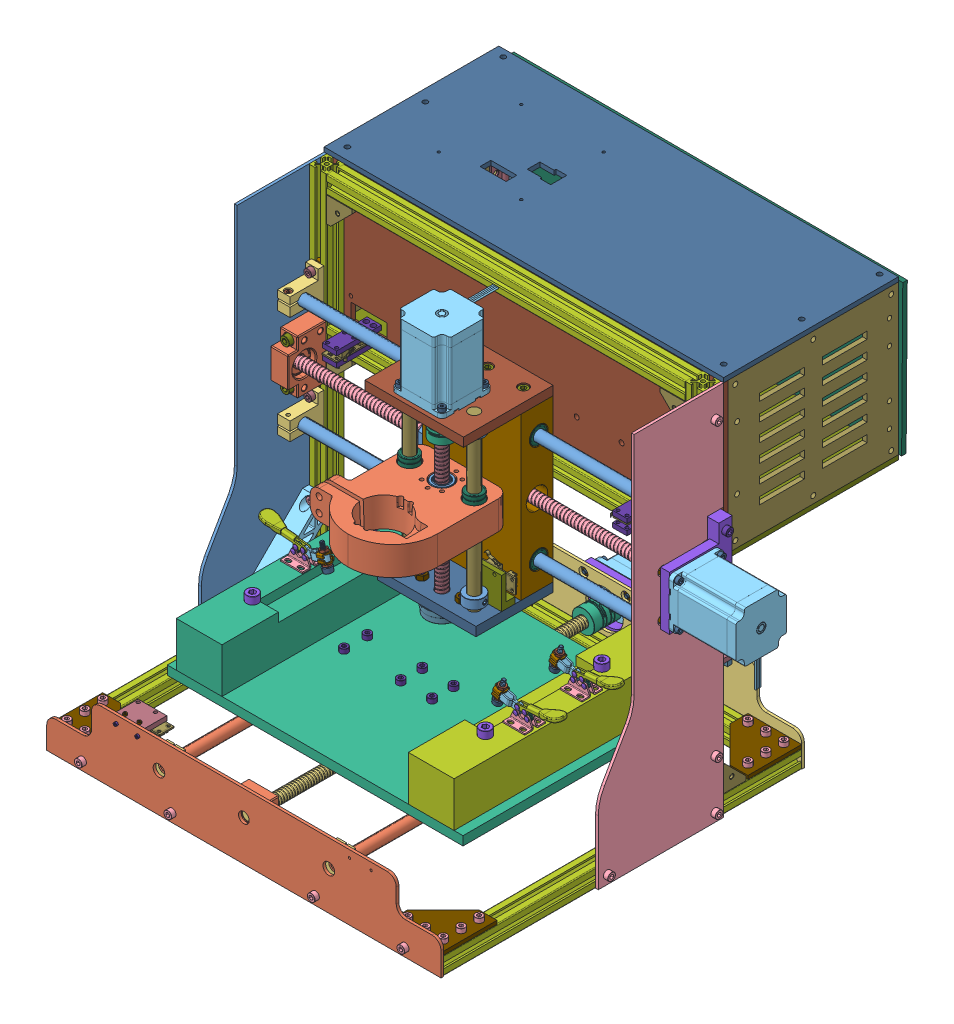
SolidWorks assembly CNC_DRILL1, configuration Default. Lengths in mm.
Overall size (538 440.9 520.73).
399 component instances, 72 part files, 0 mates.
Components (placement in the parent):
- TRuc_X(Default-_flexible1)(Default-_flexible1)-1: TRuc_X(Default-_flexible1)(Default-_flexible1) [Default] at (272.9113 10.6383 299.2443) size (530 400 73.78)
  - truc_12 - Copy(290)-2-1: truc_12 - Copy(290)-2 [Default] at (200.4373 66.1539 173.7374) x (0 0.697568 -0.716519) z (0 0.716519 0.697568) size (12 434 12)
  - truc_12 - Copy(290)-2-2: truc_12 - Copy(290)-2 [Default] at (-233.5627 186.1539 173.7374) x (0 0.783991 -0.620772) z (0 -0.620772 -0.783991) size (12 434 12)
  - BF12.step-2-1: BF12.step-2 [Default] at (-226.5627 126.1539 150.7374) x (0 -1 0) z (-1 0 0) size (60 43 20)
  - SK12.stp-2-1: SK12.stp-2 [Default] at (200.4373 207.1539 150.7374) x (-1 0 0) z (0 1 0) size (14 38 42)
  - SK12.stp-2-2: SK12.stp-2 [Default] at (-219.5627 207.1539 150.7374) x (-1 0 0) z (0 1 0) size (14 38 42)
  - SK12.stp-2-3: SK12.stp-2 [Default] at (186.4373 45.1539 150.7374) x (1 0 0) z (0 -1 0) size (14 38 42)
  - SK12.stp-2-4: SK12.stp-2 [Default] at (-233.5627 45.1539 150.7374) x (1 0 0) z (0 -1 0) size (14 38 42)
  - vitme-t8-buoc2 - Copy-2-1: vitme-t8-buoc2 - Copy-2 [Default] at (172.4373 126.1539 175.7374) x (0 0.453903 0.891051) z (-1 0 0) size (13.38 13.38 423)
  - C-57STM04-2-1: C-57STM04-2 [Default] at (218.4373 126.1539 175.7374) size (101.6 88.2 56.4)
  - GSASL25-8-12_b-2-1: GSASL25-8-12_b-2 [Default] at (204.2373 126.1539 175.7374) x (-1 0 0) z (0 0.118835 -0.992914) size (31 25.01 25.01)
  - HFS5-2020-380-2-1: HFS5-2020-380-2 [Default] at (-226.5627 -82.8461 140.7374) x (1 0 0) z (0 -1 0) size (20 20 400)
  - HFS5-2020-380-2-2: HFS5-2020-380-2 [Default] at (-196.5627 140.1539 140.7374) x (0 1 0) z (-1 0 0) size (20 20 400)
  - HFS5-2020-380-2-3: HFS5-2020-380-2 [Default] at (-196.5627 287.1539 140.7374) x (0 1 0) z (-1 0 0) size (20 20 400)
  - HFS5-2020-380-2-4: HFS5-2020-380-2 [Default] at (193.4373 -82.8461 140.7374) x (1 0 0) z (0 -1 0) size (20 20 400)
  - Part1346-2-1: Part1346-2 [Default] at (218.4373 126.1539 175.7374) x (-1 0 0) z (0 0 -1) size (15 100 70)
  - T-Nut_2020_M5.step-2-1: T-Nut_2020_M5.step-2 [Default] at (193.4373 170.1539 148.7374) size (10 10.5 5)
  - T-Nut_2020_M5.step-2-2: T-Nut_2020_M5.step-2 [Default] at (-218.5627 261.2539 140.7374) x (0 0 -1) z (1 0 0) size (10 10.5 5)
  - T-Nut_2020_M5.step-2-3: T-Nut_2020_M5.step-2 [Default] at (-218.5627 114.2539 140.7374) x (0 0 -1) z (1 0 0) size (10 10.5 5)
  - T-Nut_2020_M5.step-2-4: T-Nut_2020_M5.step-2 [Default] at (-226.5627 170.1539 148.7374) size (10 10.5 5)
  - T-Nut_2020_M5.step-2-5: T-Nut_2020_M5.step-2 [Default] at (185.4373 261.2539 140.7374) x (0 0 1) z (-1 0 0) size (10 10.5 5)
  - T-Nut_2020_M5.step-2-6: T-Nut_2020_M5.step-2 [Default] at (167.5373 279.1539 140.7374) x (0 0 -1) z (0 -1 0) size (10 10.5 5)
  - T-Nut_2020_M5.step-2-7: T-Nut_2020_M5.step-2 [Default] at (185.4373 114.2539 140.7374) x (0 0 1) z (-1 0 0) size (10 10.5 5)
  - T-Nut_2020_M5.step-2-8: T-Nut_2020_M5.step-2 [Default] at (193.4373 82.1539 148.7374) size (10 10.5 5)
  - T-Nut_2020_M5.step-2-9: T-Nut_2020_M5.step-2 [Default] at (193.4373 50.1539 148.7374) size (10 10.5 5)
  - T-Nut_2020_M5.step-2-10: T-Nut_2020_M5.step-2 [Default] at (-200.6627 279.1539 140.7374) x (0 0 -1) z (0 -1 0) size (10 10.5 5)
  - T-Nut_2020_M5.step-2-11: T-Nut_2020_M5.step-2 [Default] at (193.4373 202.1539 148.7374) size (10 10.5 5)
  - T-Nut_2020_M5.step-2-12: T-Nut_2020_M5.step-2 [Default] at (167.5373 132.1539 140.7374) x (0 0 -1) z (0 -1 0) size (10 10.5 5)
  - T-Nut_2020_M5.step-2-13: T-Nut_2020_M5.step-2 [Default] at (201.4373 86.1539 140.7374) x (0 0 -1) z (1 0 0) size (10 10.5 5)
  - T-Nut_2020_M5.step-2-14: T-Nut_2020_M5.step-2 [Default] at (201.4373 166.1539 140.7374) x (0 0 -1) z (1 0 0) size (10 10.5 5)
  - T-Nut_2020_M5.step-2-15: T-Nut_2020_M5.step-2 [Default] at (-226.5627 50.1539 148.7374) size (10 10.5 5)
  - T-Nut_2020_M5.step-2-16: T-Nut_2020_M5.step-2 [Default] at (-226.5627 202.1539 148.7374) size (10 10.5 5)
  - T-Nut_2020_M5.step-2-17: T-Nut_2020_M5.step-2 [Default] at (-226.5627 82.1539 148.7374) size (10 10.5 5)
  - T-Nut_2020_M5.step-2-18: T-Nut_2020_M5.step-2 [Default] at (-200.6627 132.1539 140.7374) x (0 0 -1) z (0 -1 0) size (10 10.5 5)
  - socket head cap screw_iso(ISO 4762 M4 x 20 - 20N)-2-1: socket head cap screw_iso(ISO 4762 M4 x 20 - 20N)-2 [Default] at (227.4373 149.7239 199.3074) x (-1 0 0) z (0 0.924225 0.381849) size (24 7 7)
  - socket head cap screw_iso(ISO 4762 M4 x 20 - 20N)-2-2: socket head cap screw_iso(ISO 4762 M4 x 20 - 20N)-2 [Default] at (227.4373 102.5839 199.3074) x (-1 0 0) z (0 0.924225 0.381849) size (24 7 7)
  - socket head cap screw_iso(ISO 4762 M4 x 20 - 20N)-2-3: socket head cap screw_iso(ISO 4762 M4 x 20 - 20N)-2 [Default] at (227.4373 102.5839 152.1674) x (-1 0 0) z (0 0.924225 0.381849) size (24 7 7)
  - socket head cap screw_iso(ISO 4762 M4 x 20 - 20N)-2-4: socket head cap screw_iso(ISO 4762 M4 x 20 - 20N)-2 [Default] at (227.4373 149.7239 152.1674) x (-1 0 0) z (0 0.924225 0.381849) size (24 7 7)
  - socket head cap screw_iso(ISO 4762 M4 x 12 - 12N)-2-1: socket head cap screw_iso(ISO 4762 M4 x 12 - 12N)-2 [Default] at (193.4373 195.1539 183.7374) x (0 -1 0) z (-0.018045 0 0.999837) size (16 7 7)
  - socket head cap screw_iso(ISO 4762 M4 x 12 - 12N)-2-2: socket head cap screw_iso(ISO 4762 M4 x 12 - 12N)-2 [Default] at (193.4373 57.1539 183.7374) x (0 1 0) z (0.474631 0 0.880185) size (16 7 7)
  - socket head cap screw_iso(ISO 4762 M4 x 12 - 12N)-2-3: socket head cap screw_iso(ISO 4762 M4 x 12 - 12N)-2 [Default] at (-226.5627 57.1539 183.7374) x (0 1 0) z (0 0 1) size (16 7 7)
  - socket head cap screw_iso(ISO 4762 M4 x 12 - 12N)-2-4: socket head cap screw_iso(ISO 4762 M4 x 12 - 12N)-2 [Default] at (-226.5627 195.1539 183.7374) x (0 -1 0) z (0.827236 0 -0.561854) size (16 7 7)
  - LBSBL6-2028-C_b-2-1: LBSBL6-2028-C_b-2 [Default] at (183.4373 130.1539 140.7374) x (0 0 1) z (0 -1 0) size (20 29.7 29.7)
  - LBSBL6-2028-C_b-2-2: LBSBL6-2028-C_b-2 [Default] at (183.4373 277.1539 140.7374) x (0 0 1) z (0 -1 0) size (20 29.7 29.7)
  - LBSBL6-2028-C_b-2-3: LBSBL6-2028-C_b-2 [Default] at (-216.5627 277.1539 140.7374) x (0 0 -1) z (0 -1 0) size (20 29.7 29.7)
  - LBSBL6-2028-C_b-2-4: LBSBL6-2028-C_b-2 [Default] at (-216.5627 130.1539 140.7374) x (0 0 -1) z (0 -1 0) size (20 29.7 29.7)
  - socket head cap screw_iso(ISO 4762 M5 x 10 - 10N)-2-1: socket head cap screw_iso(ISO 4762 M5 x 10 - 10N)-2 [Default] at (193.4373 50.1539 162.2374) x (0 0 -1) z (1 0 0) size (15 8.5 8.5)
  - socket head cap screw_iso(ISO 4762 M5 x 10 - 10N)-2-2: socket head cap screw_iso(ISO 4762 M5 x 10 - 10N)-2 [Default] at (-226.5627 82.1539 162.2374) x (0 0 -1) z (0.958405 -0.28541 0) size (15 8.5 8.5)
  - socket head cap screw_iso(ISO 4762 M5 x 10 - 10N)-2-3: socket head cap screw_iso(ISO 4762 M5 x 10 - 10N)-2 [Default] at (193.4373 82.1539 162.2374) x (0 0 -1) z (-0.921919 0.387383 0) size (15 8.5 8.5)
  - socket head cap screw_iso(ISO 4762 M5 x 10 - 10N)-2-4: socket head cap screw_iso(ISO 4762 M5 x 10 - 10N)-2 [Default] at (193.4373 202.1539 162.2374) x (0 0 -1) z (-0.991273 -0.131825 0) size (15 8.5 8.5)
  - socket head cap screw_iso(ISO 4762 M5 x 10 - 10N)-2-5: socket head cap screw_iso(ISO 4762 M5 x 10 - 10N)-2 [Default] at (-226.5627 170.1539 162.2374) x (0 0 -1) z (0.309145 -0.951015 0) size (15 8.5 8.5)
  - socket head cap screw_iso(ISO 4762 M5 x 10 - 10N)-2-6: socket head cap screw_iso(ISO 4762 M5 x 10 - 10N)-2 [Default] at (-226.5627 202.1539 162.2374) x (0 0 -1) z (0.089609 0.995977 0) size (15 8.5 8.5)
  - socket head cap screw_iso(ISO 4762 M5 x 10 - 10N)-2-7: socket head cap screw_iso(ISO 4762 M5 x 10 - 10N)-2 [Default] at (-226.5627 50.1539 162.2374) x (0 0 -1) z (1 0 0) size (15 8.5 8.5)
  - socket head cap screw_iso(ISO 4762 M5 x 10 - 10N)-2-8: socket head cap screw_iso(ISO 4762 M5 x 10 - 10N)-2 [Default] at (193.4373 170.1539 162.2374) x (0 0 -1) z (-0.808147 -0.58898 0) size (15 8.5 8.5)
  - socket head cap screw_iso(ISO 4762 M4 x 8 - 8N)-2-1: socket head cap screw_iso(ISO 4762 M4 x 8 - 8N)-2 [Default] at (-208.5627 114.2539 140.7374) x (-1 0 0) z (0 -0.835631 0.549291) size (12 7 7)
  - socket head cap screw_iso(ISO 4762 M4 x 8 - 8N)-2-2: socket head cap screw_iso(ISO 4762 M4 x 8 - 8N)-2 [Default] at (-208.5627 261.2539 140.7374) x (-1 0 0) z (0 0.928406 0.371567) size (12 7 7)
  - socket head cap screw_iso(ISO 4762 M4 x 8 - 8N)-2-3: socket head cap screw_iso(ISO 4762 M4 x 8 - 8N)-2 [Default] at (-200.6627 122.1539 140.7374) x (0 1 0) z (-0.53836 0 0.842715) size (12 7 7)
  - socket head cap screw_iso(ISO 4762 M4 x 8 - 8N)-2-4: socket head cap screw_iso(ISO 4762 M4 x 8 - 8N)-2 [Default] at (167.5373 122.1539 140.7374) x (0 1 0) z (0 0 1) size (12 7 7)
  - socket head cap screw_iso(ISO 4762 M4 x 8 - 8N)-2-5: socket head cap screw_iso(ISO 4762 M4 x 8 - 8N)-2 [Default] at (167.5373 269.1539 140.7374) x (0 1 0) z (0 0 1) size (12 7 7)
  - socket head cap screw_iso(ISO 4762 M4 x 8 - 8N)-2-6: socket head cap screw_iso(ISO 4762 M4 x 8 - 8N)-2 [Default] at (-200.6627 269.1539 140.7374) x (0 1 0) z (0 0 1) size (12 7 7)
  - socket head cap screw_iso(ISO 4762 M4 x 8 - 8N)-2-7: socket head cap screw_iso(ISO 4762 M4 x 8 - 8N)-2 [Default] at (175.4373 261.2539 140.7374) x (1 0 0) z (0 0.276048 0.961144) size (12 7 7)
  - socket head cap screw_iso(ISO 4762 M4 x 8 - 8N)-2-8: socket head cap screw_iso(ISO 4762 M4 x 8 - 8N)-2 [Default] at (175.4373 114.2539 140.7374) x (1 0 0) z (0 -0.200046 0.979787) size (12 7 7)
  - T-Nut_2020_M6.step-2-1: T-Nut_2020_M6.step-2 [Default] at (-226.5627 149.1539 148.7374) size (10 10.5 5)
  - T-Nut_2020_M6.step-2-2: T-Nut_2020_M6.step-2 [Default] at (-226.5627 103.1539 148.7374) size (10 10.5 5)
  - socket head cap screw_iso(ISO 4762 M6 x 35 - 24N)-2-1: socket head cap screw_iso(ISO 4762 M6 x 35 - 24N)-2 [Default] at (-226.5627 103.1539 187.7374) x (0 0 -1) z (1 0 0) size (41 10 10)
  - socket head cap screw_iso(ISO 4762 M6 x 35 - 24N)-2-2: socket head cap screw_iso(ISO 4762 M6 x 35 - 24N)-2 [Default] at (-226.5627 149.1539 187.7374) x (0 0 -1) z (0.254319 -0.96712 0) size (41 10 10)
  - socket head cap screw_iso(ISO 4762 M5 x 20 - 20N)-2-1: socket head cap screw_iso(ISO 4762 M5 x 20 - 20N)-2 [Default] at (223.4373 86.1539 140.7374) x (-1 0 0) z (0 0.924225 0.381849) size (25 8.5 8.5)
  - socket head cap screw_iso(ISO 4762 M5 x 20 - 20N)-2-2: socket head cap screw_iso(ISO 4762 M5 x 20 - 20N)-2 [Default] at (223.4373 166.1539 140.7374) x (-1 0 0) z (0 0.924225 0.381849) size (25 8.5 8.5)
  - hex nut style 1 gradeab_iso(ISO - 4032 - M4 - W - N)-2-1: hex nut style 1 gradeab_iso(ISO - 4032 - M4 - W - N)-2 [Default] at (205.2373 102.5839 199.3074) x (0 0.3952 0.918595) z (-1 0 0) size (7 8.08 3.2)
  - hex nut style 1 gradeab_iso(ISO - 4032 - M4 - W - N)-2-2: hex nut style 1 gradeab_iso(ISO - 4032 - M4 - W - N)-2 [Default] at (205.2373 149.7239 199.3074) x (0 0.883759 0.467943) z (-1 0 0) size (7 8.08 3.2)
  - hex nut style 1 gradeab_iso(ISO - 4032 - M4 - W - N)-2-3: hex nut style 1 gradeab_iso(ISO - 4032 - M4 - W - N)-2 [Default] at (205.2373 149.7239 152.1674) x (0 0.570691 0.821165) z (-1 0 0) size (7 8.08 3.2)
  - hex nut style 1 gradeab_iso(ISO - 4032 - M4 - W - N)-2-4: hex nut style 1 gradeab_iso(ISO - 4032 - M4 - W - N)-2 [Default] at (205.2373 102.5839 152.1674) x (0 0.587281 0.809383) z (-1 0 0) size (7 8.08 3.2)
  - _sfu1204 nut-2-1: _sfu1204 nut-2 [Default] at (-74.9814 126.1539 175.7374) x (0 0 -1) z (0 -1 0) size (30 35 40.5)
- Truc_y(Default-_flexible1)(Default-_flexible1)-1: Truc_y(Default-_flexible1)(Default-_flexible1) [Default] at (445.7091 -502.2078 538.5872) size (440 90 490)
  - BF12.step-2-1: BF12.step-2 [Default] at (-189.1104 410 191.3946) size (60 43 20)
  - SK12.stp-2-1: SK12.stp-2 [Default] at (-305.1104 410 -195.6054) x (0 0 1) z (-1 0 0) size (14 38 42)
  - SK12.stp-2-2: SK12.stp-2 [Default] at (-73.1104 410 198.3946) x (0 0 -1) z (1 0 0) size (14 38 42)
  - SK12.stp-2-3: SK12.stp-2 [Default] at (-305.1104 410 184.3946) x (0 0 1) z (-1 0 0) size (14 38 42)
  - SK12.stp-2-4: SK12.stp-2 [Default] at (-73.1104 410 -181.6054) x (0 0 -1) z (1 0 0) size (14 38 42)
  - C-57STM04-2-1: C-57STM04-2 [Default] at (-189.1104 435 -213.6054) x (0 0 -1) z (1 0 0) size (101.6 88.2 56.4)
  - GSASL25-8-12_b-2-1: GSASL25-8-12_b-2 [Default] at (-189.1104 435 -205.6054) x (0 0 1) z (-0.696455 -0.717601 0) size (31 25.01 25.01)
  - HFS5-2020-380-2-1: HFS5-2020-380-2 [Default] at (-9.3604 400 191.3946) x (0 -1 0) z (1 0 0) size (20 20 400)
  - HFS5-2020-380-2-2: HFS5-2020-380-2 [Default] at (-399.3604 400 181.3946) size (20 20 400)
  - HFS5-2020-380-2-3: HFS5-2020-380-2 [Default] at (20.6396 400 181.3946) size (20 20 400)
  - HFS5-2020-380-2-4: HFS5-2020-380-2 [Default] at (-9.3604 400 -188.6054) x (0 -1 0) z (1 0 0) size (20 20 400)
  - Part1346-2-1: Part1346-2 [Default] at (-189.1104 435 -213.6054) x (0 0 1) z (0 -1 0) size (15 100 70)
  - T-Nut_2020_M5.step-2-1: T-Nut_2020_M5.step-2 [Default] at (-391.3604 400 165.4946) x (0 -1 0) z (1 0 0) size (10 10.5 5)
  - T-Nut_2020_M5.step-2-2: T-Nut_2020_M5.step-2 [Default] at (12.6396 400 165.4946) x (0 -1 0) z (-1 0 0) size (10 10.5 5)
  - T-Nut_2020_M5.step-2-3: T-Nut_2020_M5.step-2 [Default] at (-110.1104 408 -188.6054) x (0 0 -1) z (0 1 0) size (10 10.5 5)
  - T-Nut_2020_M5.step-2-4: T-Nut_2020_M5.step-2 [Default] at (-300.1104 408 191.3946) x (0 0 -1) z (0 1 0) size (10 10.5 5)
  - T-Nut_2020_M5.step-2-5: T-Nut_2020_M5.step-2 [Default] at (-78.1104 408 -188.6054) x (0 0 -1) z (0 1 0) size (10 10.5 5)
  - T-Nut_2020_M5.step-2-6: T-Nut_2020_M5.step-2 [Default] at (-110.1104 408 191.3946) x (0 0 -1) z (0 1 0) size (10 10.5 5)
  - T-Nut_2020_M5.step-2-7: T-Nut_2020_M5.step-2 [Default] at (-300.1104 408 -188.6054) x (0 0 -1) z (0 1 0) size (10 10.5 5)
  - T-Nut_2020_M5.step-2-8: T-Nut_2020_M5.step-2 [Default] at (12.6396 400 -162.7054) x (0 1 0) z (-1 0 0) size (10 10.5 5)
  - T-Nut_2020_M5.step-2-9: T-Nut_2020_M5.step-2 [Default] at (-373.4604 400 -180.6054) x (0 -1 0) z (0 0 1) size (10 10.5 5)
  - T-Nut_2020_M5.step-2-10: T-Nut_2020_M5.step-2 [Default] at (-5.2604 400 -180.6054) x (0 1 0) z (0 0 1) size (10 10.5 5)
  - T-Nut_2020_M5.step-2-11: T-Nut_2020_M5.step-2 [Default] at (-5.2604 400 183.3946) x (0 -1 0) z (0 0 -1) size (10 10.5 5)
  - T-Nut_2020_M5.step-2-12: T-Nut_2020_M5.step-2 [Default] at (-149.1104 400 -196.6054) x (0 -1 0) z (0 0 -1) size (10 10.5 5)
  - T-Nut_2020_M5.step-2-13: T-Nut_2020_M5.step-2 [Default] at (-268.1104 408 -188.6054) x (0 0 1) z (0 1 0) size (10 10.5 5)
  - T-Nut_2020_M5.step-2-14: T-Nut_2020_M5.step-2 [Default] at (-268.1104 408 191.3946) x (0 0 -1) z (0 1 0) size (10 10.5 5)
  - T-Nut_2020_M5.step-2-15: T-Nut_2020_M5.step-2 [Default] at (-373.4604 400 183.3946) x (0 -1 0) z (0 0 -1) size (10 10.5 5)
  - T-Nut_2020_M5.step-2-16: T-Nut_2020_M5.step-2 [Default] at (-229.1104 400 -196.6054) x (0 1 0) z (0 0 -1) size (10 10.5 5)
  - T-Nut_2020_M5.step-2-17: T-Nut_2020_M5.step-2 [Default] at (-391.3604 400 -162.7054) x (0 1 0) z (1 0 0) size (10 10.5 5)
  - T-Nut_2020_M5.step-2-18: T-Nut_2020_M5.step-2 [Default] at (-78.1104 408 191.3946) x (0 0 -1) z (0 1 0) size (10 10.5 5)
  - socket head cap screw_iso(ISO 4762 M4 x 20 - 20N)-2-1: socket head cap screw_iso(ISO 4762 M4 x 20 - 20N)-2 [Default] at (-165.5404 458.57 -222.6054) x (0 0 1) z (-1 0 0) size (24 7 7)
  - socket head cap screw_iso(ISO 4762 M4 x 20 - 20N)-2-2: socket head cap screw_iso(ISO 4762 M4 x 20 - 20N)-2 [Default] at (-212.6804 411.43 -222.6054) x (0 0 1) z (-1 0 0) size (24 7 7)
  - socket head cap screw_iso(ISO 4762 M4 x 20 - 20N)-2-3: socket head cap screw_iso(ISO 4762 M4 x 20 - 20N)-2 [Default] at (-165.5404 411.43 -222.6054) x (0 0 1) z (-1 0 0) size (24 7 7)
  - socket head cap screw_iso(ISO 4762 M4 x 20 - 20N)-2-4: socket head cap screw_iso(ISO 4762 M4 x 20 - 20N)-2 [Default] at (-212.6804 458.57 -222.6054) x (0 0 1) z (-1 0 0) size (24 7 7)
  - socket head cap screw_iso(ISO 4762 M4 x 12 - 12N)-2-1: socket head cap screw_iso(ISO 4762 M4 x 12 - 12N)-2 [Default] at (-293.1104 443 191.3946) size (16 7 7)
  - socket head cap screw_iso(ISO 4762 M4 x 12 - 12N)-2-2: socket head cap screw_iso(ISO 4762 M4 x 12 - 12N)-2 [Default] at (-293.1104 443 -188.6054) size (16 7 7)
  - socket head cap screw_iso(ISO 4762 M4 x 12 - 12N)-2-3: socket head cap screw_iso(ISO 4762 M4 x 12 - 12N)-2 [Default] at (-85.1104 443 -188.6054) x (-1 0 0) z (0 -0.924225 -0.381849) size (16 7 7)
  - socket head cap screw_iso(ISO 4762 M4 x 12 - 12N)-2-4: socket head cap screw_iso(ISO 4762 M4 x 12 - 12N)-2 [Default] at (-85.1104 443 191.3946) x (-1 0 0) z (0 0.904309 -0.426879) size (16 7 7)
  - LBSBL6-2028-C_b-2-1: LBSBL6-2028-C_b-2 [Default] at (-389.3604 400 181.3946) x (0 -1 0) z (1 0 0) size (20 29.7 29.7)
  - LBSBL6-2028-C_b-2-2: LBSBL6-2028-C_b-2 [Default] at (10.6396 400 -178.6054) x (0 -1 0) z (-1 0 0) size (20 29.7 29.7)
  - LBSBL6-2028-C_b-2-3: LBSBL6-2028-C_b-2 [Default] at (10.6396 400 181.3946) x (0 -1 0) z (0 0 -1) size (20 29.7 29.7)
  - LBSBL6-2028-C_b-2-4: LBSBL6-2028-C_b-2 [Default] at (-389.3604 400 -178.6054) x (0 1 0) z (1 0 0) size (20 29.7 29.7)
  - socket head cap screw_iso(ISO 4762 M5 x 10 - 10N)-2-1: socket head cap screw_iso(ISO 4762 M5 x 10 - 10N)-2 [Default] at (-110.1104 421.5 -188.6054) x (0 -1 0) z (0 0 1) size (15 8.5 8.5)
  - socket head cap screw_iso(ISO 4762 M5 x 10 - 10N)-2-2: socket head cap screw_iso(ISO 4762 M5 x 10 - 10N)-2 [Default] at (-78.1104 421.5 -188.6054) x (0 -1 0) z (0 0 1) size (15 8.5 8.5)
  - socket head cap screw_iso(ISO 4762 M5 x 10 - 10N)-2-3: socket head cap screw_iso(ISO 4762 M5 x 10 - 10N)-2 [Default] at (-300.1104 421.5 -188.6054) x (0 -1 0) z (0 0 1) size (15 8.5 8.5)
  - socket head cap screw_iso(ISO 4762 M5 x 10 - 10N)-2-4: socket head cap screw_iso(ISO 4762 M5 x 10 - 10N)-2 [Default] at (-78.1104 421.5 191.3946) x (0 -1 0) z (0 0 1) size (15 8.5 8.5)
  - socket head cap screw_iso(ISO 4762 M5 x 10 - 10N)-2-5: socket head cap screw_iso(ISO 4762 M5 x 10 - 10N)-2 [Default] at (-268.1104 421.5 191.3946) x (0 -1 0) z (0.36092 0 0.932597) size (15 8.5 8.5)
  - socket head cap screw_iso(ISO 4762 M5 x 10 - 10N)-2-6: socket head cap screw_iso(ISO 4762 M5 x 10 - 10N)-2 [Default] at (-110.1104 421.5 191.3946) x (0 -1 0) z (0 0 1) size (15 8.5 8.5)
  - socket head cap screw_iso(ISO 4762 M5 x 10 - 10N)-2-7: socket head cap screw_iso(ISO 4762 M5 x 10 - 10N)-2 [Default] at (-268.1104 421.5 -188.6054) x (0 -1 0) z (0 0 1) size (15 8.5 8.5)
  - socket head cap screw_iso(ISO 4762 M5 x 10 - 10N)-2-8: socket head cap screw_iso(ISO 4762 M5 x 10 - 10N)-2 [Default] at (-300.1104 421.5 191.3946) x (0 -1 0) z (0.994997 0 -0.09991) size (15 8.5 8.5)
  - T-Nut_2020_M6.step-2-1: T-Nut_2020_M6.step-2 [Default] at (-166.1104 408 191.3946) x (0 0 1) z (0 1 0) size (10 10.5 5)
  - T-Nut_2020_M6.step-2-2: T-Nut_2020_M6.step-2 [Default] at (-212.1104 408 191.3946) x (0 0 -1) z (0 1 0) size (10 10.5 5)
  - socket head cap screw_iso(ISO 4762 M6 x 35 - 24N)-2-1: socket head cap screw_iso(ISO 4762 M6 x 35 - 24N)-2 [Default] at (-212.1104 447 191.3946) x (0 -1 0) z (0.832998 0 -0.553276) size (41 10 10)
  - socket head cap screw_iso(ISO 4762 M6 x 35 - 24N)-2-2: socket head cap screw_iso(ISO 4762 M6 x 35 - 24N)-2 [Default] at (-166.1104 447 191.3946) x (0 -1 0) z (0.794116 0 -0.607766) size (41 10 10)
  - socket head cap screw_iso(ISO 4762 M5 x 20 - 20N)-2-1: socket head cap screw_iso(ISO 4762 M5 x 20 - 20N)-2 [Default] at (-206.6104 465 -12.4264) x (0 -1 0) z (0 0 1) size (25 8.5 8.5)
  - socket head cap screw_iso(ISO 4762 M5 x 20 - 20N)-2-2: socket head cap screw_iso(ISO 4762 M5 x 20 - 20N)-2 [Default] at (-229.1104 400 -218.6054) x (0 0 1) z (-1 0 0) size (25 8.5 8.5)
  - socket head cap screw_iso(ISO 4762 M5 x 20 - 20N)-2-3: socket head cap screw_iso(ISO 4762 M5 x 20 - 20N)-2 [Default] at (-299.3604 465 12.5736) x (0 -1 0) z (0 0 1) size (25 8.5 8.5)
  - socket head cap screw_iso(ISO 4762 M5 x 20 - 20N)-2-4: socket head cap screw_iso(ISO 4762 M5 x 20 - 20N)-2 [Default] at (-299.3604 465 -13.4264) x (0 -1 0) z (0 0 1) size (25 8.5 8.5)
  - socket head cap screw_iso(ISO 4762 M5 x 20 - 20N)-2-5: socket head cap screw_iso(ISO 4762 M5 x 20 - 20N)-2 [Default] at (-109.3604 465 -13.4264) x (0 -1 0) z (0 0 1) size (25 8.5 8.5)
  - socket head cap screw_iso(ISO 4762 M5 x 20 - 20N)-2-6: socket head cap screw_iso(ISO 4762 M5 x 20 - 20N)-2 [Default] at (-78.8604 465 -13.4264) x (0 -1 0) z (0 0 1) size (25 8.5 8.5)
  - socket head cap screw_iso(ISO 4762 M5 x 20 - 20N)-2-7: socket head cap screw_iso(ISO 4762 M5 x 20 - 20N)-2 [Default] at (-109.3604 465 12.5736) x (0 -1 0) z (0 0 1) size (25 8.5 8.5)
  - socket head cap screw_iso(ISO 4762 M5 x 20 - 20N)-2-8: socket head cap screw_iso(ISO 4762 M5 x 20 - 20N)-2 [Default] at (-268.8604 465 12.5736) x (0 -1 0) z (0 0 1) size (25 8.5 8.5)
  - socket head cap screw_iso(ISO 4762 M5 x 20 - 20N)-2-9: socket head cap screw_iso(ISO 4762 M5 x 20 - 20N)-2 [Default] at (-171.6104 465 11.5736) x (0 -1 0) z (-0.093588 0 0.995611) size (25 8.5 8.5)
  - socket head cap screw_iso(ISO 4762 M5 x 20 - 20N)-2-10: socket head cap screw_iso(ISO 4762 M5 x 20 - 20N)-2 [Default] at (-171.6104 465 -12.4264) x (0 -1 0) z (0 0 1) size (25 8.5 8.5)
  - socket head cap screw_iso(ISO 4762 M5 x 20 - 20N)-2-11: socket head cap screw_iso(ISO 4762 M5 x 20 - 20N)-2 [Default] at (-268.8604 465 -13.4264) x (0 -1 0) z (0 0 1) size (25 8.5 8.5)
  - socket head cap screw_iso(ISO 4762 M5 x 20 - 20N)-2-12: socket head cap screw_iso(ISO 4762 M5 x 20 - 20N)-2 [Default] at (-149.1104 400 -218.6054) x (0 0 1) z (-0.939203 -0.343361 0) size (25 8.5 8.5)
  - socket head cap screw_iso(ISO 4762 M5 x 20 - 20N)-2-13: socket head cap screw_iso(ISO 4762 M5 x 20 - 20N)-2 [Default] at (-78.8604 465 12.5736) x (0 -1 0) z (0 0 1) size (25 8.5 8.5)
  - socket head cap screw_iso(ISO 4762 M5 x 20 - 20N)-2-14: socket head cap screw_iso(ISO 4762 M5 x 20 - 20N)-2 [Default] at (-206.6104 465 11.5736) x (0 -1 0) z (0 0 1) size (25 8.5 8.5)
  - hex nut style 1 gradeab_iso(ISO - 4032 - M4 - W - N)-2-1: hex nut style 1 gradeab_iso(ISO - 4032 - M4 - W - N)-2 [Default] at (-165.5404 458.57 -203.6054) x (-0.923728 -0.383049 0) z (0 0 -1) size (7 8.08 3.2)
  - hex nut style 1 gradeab_iso(ISO - 4032 - M4 - W - N)-2-2: hex nut style 1 gradeab_iso(ISO - 4032 - M4 - W - N)-2 [Default] at (-212.6804 458.57 -203.6054) x (-0.923728 -0.383049 0) z (0 0 -1) size (7 8.08 3.2)
  - hex nut style 1 gradeab_iso(ISO - 4032 - M4 - W - N)-2-3: hex nut style 1 gradeab_iso(ISO - 4032 - M4 - W - N)-2 [Default] at (-165.5404 411.43 -203.6054) x (-0.923728 -0.383049 0) z (0 0 -1) size (7 8.08 3.2)
  - hex nut style 1 gradeab_iso(ISO - 4032 - M4 - W - N)-2-4: hex nut style 1 gradeab_iso(ISO - 4032 - M4 - W - N)-2 [Default] at (-212.6804 411.43 -200.4054) size (7 8.08 3.2)
  - _sfu1204 nut-2-1: _sfu1204 nut-2 [Default] at (-189.1104 435 25.5736) x (0 -1 0) z (1 0 0) size (30 35 40.5)
  - truc_12(290)-1: truc_12(290) [Default] at (-94.1104 433 -195.6054) x (0.897653 0.440702 0) z (0.440702 -0.897653 0) size (12 394 12)
  - truc_12(290)-2: truc_12(290) [Default] at (-284.1104 433 -195.6054) x (-0.996768 0.080336 0) z (0.080336 0.996768 0) size (12 394 12)
  - vitme-t8-buoc2-1: vitme-t8-buoc2 [Default] at (-189.1104 435 185.5946) x (-0.966282 0.257487 0) z (0 0 -1) size (13.38 13.38 385)
  - socket head cap screw_iso(ISO 4762 M5 x 8 - 8N)-1: socket head cap screw_iso(ISO 4762 M5 x 8 - 8N) [Default] at (-5.2604 400 172.3946) x (0 0 1) z (0.936297 0.351211 0) size (13 8.5 8.5)
  - socket head cap screw_iso(ISO 4762 M5 x 8 - 8N)-2: socket head cap screw_iso(ISO 4762 M5 x 8 - 8N) [Default] at (-373.4604 400 -169.6054) x (0 0 -1) z (0.965623 0.259948 0) size (13 8.5 8.5)
  - socket head cap screw_iso(ISO 4762 M5 x 8 - 8N)-3: socket head cap screw_iso(ISO 4762 M5 x 8 - 8N) [Default] at (-5.2604 400 -169.6054) x (0 0 -1) z (-0.546843 -0.837235 0) size (13 8.5 8.5)
  - socket head cap screw_iso(ISO 4762 M5 x 8 - 8N)-4: socket head cap screw_iso(ISO 4762 M5 x 8 - 8N) [Default] at (1.6396 400 165.4946) x (1 0 0) z (0 -0.486659 -0.873592) size (13 8.5 8.5)
  - socket head cap screw_iso(ISO 4762 M5 x 8 - 8N)-5: socket head cap screw_iso(ISO 4762 M5 x 8 - 8N) [Default] at (-373.4604 400 172.3946) x (0 0 1) z (0.163239 -0.986587 0) size (13 8.5 8.5)
  - socket head cap screw_iso(ISO 4762 M5 x 8 - 8N)-6: socket head cap screw_iso(ISO 4762 M5 x 8 - 8N) [Default] at (1.6396 400 -162.7054) x (1 0 0) z (0 0.347394 0.937719) size (13 8.5 8.5)
  - socket head cap screw_iso(ISO 4762 M5 x 8 - 8N)-7: socket head cap screw_iso(ISO 4762 M5 x 8 - 8N) [Default] at (-380.3604 400 165.4946) x (-1 0 0) z (0 0.976551 0.215285) size (13 8.5 8.5)
  - socket head cap screw_iso(ISO 4762 M5 x 8 - 8N)-8: socket head cap screw_iso(ISO 4762 M5 x 8 - 8N) [Default] at (-380.3604 400 -162.7054) x (-1 0 0) z (0 -0.279704 0.960086) size (13 8.5 8.5)
  - CHINA_Housing D22mm for ballscrew nut SFU1204.stp-1: CHINA_Housing D22mm for ballscrew nut SFU1204.stp [Default] at (-189.1104 435 -0.4264) x (1 0 0) z (0 1 0) size (50 36 30)
  - tamde-1: tamde [Default] at (-189.1104 450 -0.4264) x (0 1 0) z (1 0 0) size (10.45 250 330)
  - socket head cap screw_iso(ISO 4762 M4 x 16 - 16N)-1: socket head cap screw_iso(ISO 4762 M4 x 16 - 16N) [Default] at (-205.1104 435 29.5736) x (0 0 -1) z (1 0 0) size (20 7 7)
  - socket head cap screw_iso(ISO 4762 M4 x 16 - 16N)-2: socket head cap screw_iso(ISO 4762 M4 x 16 - 16N) [Default] at (-173.1104 435 29.5736) x (0 0 -1) z (1 0 0) size (20 7 7)
  - socket head cap screw_iso(ISO 4762 M4 x 16 - 16N)-3: socket head cap screw_iso(ISO 4762 M4 x 16 - 16N) [Default] at (-200.4241 423.6863 29.5736) x (0 0 -1) z (1 0 0) size (20 7 7)
  - socket head cap screw_iso(ISO 4762 M4 x 16 - 16N)-4: socket head cap screw_iso(ISO 4762 M4 x 16 - 16N) [Default] at (-200.4241 446.3137 29.5736) x (0 0 -1) z (1 0 0) size (20 7 7)
  - socket head cap screw_iso(ISO 4762 M4 x 16 - 16N)-5: socket head cap screw_iso(ISO 4762 M4 x 16 - 16N) [Default] at (-177.7967 446.3137 29.5736) x (0 0 -1) z (1 0 0) size (20 7 7)
  - socket head cap screw_iso(ISO 4762 M4 x 16 - 16N)-6: socket head cap screw_iso(ISO 4762 M4 x 16 - 16N) [Default] at (-177.7967 423.6863 29.5736) x (0 0 -1) z (1 0 0) size (20 7 7)
  - SCS12UU-1: SCS12UU [Default] at (-94.1104 433 -0.4264) size (42 28 36)
  - SCS12UU-2: SCS12UU [Default] at (-284.1104 433 -0.4264) size (42 28 36)
- TRUC_Z(Default-_flexible1)(Default-_flexible1)-1: TRUC_Z(Default-_flexible1)(Default-_flexible1) [Default] at (102.902 107.7944 426.5045) size (125 292 174)
  - C-57STM04-2-1: C-57STM04-2 [Default] at (158.0279 130.8978 99.4773) x (0 1 0) z (1 0 0) size (101.6 88.2 56.4)
  - GSASL25-8-12_b-2-1: GSASL25-8-12_b-2 [Default] at (158.0279 117.6978 99.4773) x (0 -1 0) z (0.978388 0 -0.206778) size (31 25.01 25.01)
  - socket head cap screw_iso(ISO 4762 M4 x 20 - 20N)-2-1: socket head cap screw_iso(ISO 4762 M4 x 20 - 20N)-2 [Default] at (134.4579 139.8978 75.9073) x (0 -1 0) z (0 0 1) size (24 7 7)
  - socket head cap screw_iso(ISO 4762 M4 x 20 - 20N)-2-2: socket head cap screw_iso(ISO 4762 M4 x 20 - 20N)-2 [Default] at (181.5979 139.8978 123.0473) x (0 -1 0) z (0 0 1) size (24 7 7)
  - socket head cap screw_iso(ISO 4762 M4 x 20 - 20N)-2-3: socket head cap screw_iso(ISO 4762 M4 x 20 - 20N)-2 [Default] at (181.5979 139.8978 75.9073) x (0 -1 0) z (0 0 1) size (24 7 7)
  - socket head cap screw_iso(ISO 4762 M4 x 20 - 20N)-2-4: socket head cap screw_iso(ISO 4762 M4 x 20 - 20N)-2 [Default] at (134.4579 139.8978 123.0473) x (0 -1 0) z (0 0 1) size (24 7 7)
  - hex nut style 1 gradeab_iso(ISO - 4032 - M4 - W - N)-2-1: hex nut style 1 gradeab_iso(ISO - 4032 - M4 - W - N)-2 [Default] at (181.5979 116.0978 123.0473) x (1 0 0) z (0 -1 0) size (7 8.08 3.2)
  - hex nut style 1 gradeab_iso(ISO - 4032 - M4 - W - N)-2-2: hex nut style 1 gradeab_iso(ISO - 4032 - M4 - W - N)-2 [Default] at (181.5979 116.0978 75.9073) x (1 0 0) z (0 -1 0) size (7 8.08 3.2)
  - hex nut style 1 gradeab_iso(ISO - 4032 - M4 - W - N)-2-3: hex nut style 1 gradeab_iso(ISO - 4032 - M4 - W - N)-2 [Default] at (134.4579 116.0978 123.0473) x (1 0 0) z (0 -1 0) size (7 8.08 3.2)
  - hex nut style 1 gradeab_iso(ISO - 4032 - M4 - W - N)-2-4: hex nut style 1 gradeab_iso(ISO - 4032 - M4 - W - N)-2 [Default] at (134.4579 116.0978 75.9073) x (1 0 0) z (0 -1 0) size (7 8.08 3.2)
  - _sfu1204 nut-2-1: _sfu1204 nut-2 [Default] at (158.0279 10.2978 99.4773) size (30 35 40.5)
  - socket head cap screw_iso(ISO 4762 M4 x 16 - 16N)-1: socket head cap screw_iso(ISO 4762 M4 x 16 - 16N) [Default] at (158.0279 -1.6812 83.4773) x (0 1 0) z (-0.23742 0 0.971407) size (20 7 7)
  - trucz_1-1: trucz_1 [Default] at (213.0279 -70.7022 30.4773) size (110 180 36)
  - Part1Z_BOT-1: Part1Z_BOT [Default] at (158.0279 -70.7022 73.4773) x (1 0 0) z (0 1 0) size (110 86 10)
  - Part1Z_TOP-1: Part1Z_TOP [Default] at (158.0279 129.2978 80.4773) x (-1 0 0) z (0 -1 0) size (110 100 10)
  - Assem121-1: Assem121 [Default] at (194.0279 -73.7022 99.4773) x (-0.200626 0 0.979668) z (-0.979668 0 -0.200626) size (12 203 12)
  - Assem121-2: Assem121 [Default] at (122.0279 -73.7022 99.4773) size (12 203 12)
  - vitme-t8-buoc2_trucz-1: vitme-t8-buoc2_trucz [Default] at (158.0279 89.6978 99.4773) x (0.880345 0 -0.474335) z (0 -1 0) size (12.42 12.42 180)
  - KLF000-1: KLF000 [Default] at (158.0279 -70.7022 99.4773) x (1 0 0) z (0 0 -1) size (60 15.41 36)
  - LMK12-1: LMK12 [Default] at (198.0279 -31.0022 46.4773) size (30 19 19)
  - LMK12-2: LMK12 [Default] at (118.0279 -31.0022 46.4773) size (30 19 19)
  - LMK12-3: LMK12 [Default] at (194.0279 38.2978 99.4773) x (0 -1 0) z (0.795487 0 0.60597) size (30 19 19)
  - LMK12-4: LMK12 [Default] at (122.0279 38.2978 99.4773) x (0 1 0) z (-0.335818 0 0.941927) size (30 19 19)
  - LMK12-5: LMK12 [Default] at (118.0279 88.9978 46.4773) size (30 19 19)
  - LMK12-6: LMK12 [Default] at (198.0279 88.9978 46.4773) size (30 19 19)
  - socket head cap screw_iso(ISO 4762 M6 x 16 - 16N)-1: socket head cap screw_iso(ISO 4762 M6 x 16 - 16N) [Default] at (158.0279 -70.7022 48.4773) x (0 1 0) z (0 0 1) size (22 10 10)
  - socket head cap screw_iso(ISO 4762 M6 x 16 - 16N)-2: socket head cap screw_iso(ISO 4762 M6 x 16 - 16N) [Default] at (118.0279 -70.7022 48.4773) x (0 1 0) z (0 0 1) size (22 10 10)
  - socket head cap screw_iso(ISO 4762 M6 x 16 - 16N)-3: socket head cap screw_iso(ISO 4762 M6 x 16 - 16N) [Default] at (198.0279 -70.7022 48.4773) x (0 1 0) z (0 0 1) size (22 10 10)
  - socket head cap screw_iso(ISO 4762 M6 x 16 - 16N)-4: socket head cap screw_iso(ISO 4762 M6 x 16 - 16N) [Default] at (118.0279 128.2978 48.4773) x (0 -1 0) z (0 0 1) size (22 10 10)
  - socket head cap screw_iso(ISO 4762 M6 x 16 - 16N)-5: socket head cap screw_iso(ISO 4762 M6 x 16 - 16N) [Default] at (198.0279 128.2978 48.4773) x (0 -1 0) z (0 0 1) size (22 10 10)
  - socket head cap screw_iso(ISO 4762 M6 x 16 - 16N)-6: socket head cap screw_iso(ISO 4762 M6 x 16 - 16N) [Default] at (158.0279 128.2978 48.4773) x (0 -1 0) z (0 0 1) size (22 10 10)
  - socket head cap screw_iso(ISO 4762 M6 x 20 - 20N)-1: socket head cap screw_iso(ISO 4762 M6 x 20 - 20N) [Default] at (135.5279 -82.2022 99.4773) x (0 1 0) z (0 0 1) size (26 10 10)
  - socket head cap screw_iso(ISO 4762 M6 x 20 - 20N)-2: socket head cap screw_iso(ISO 4762 M6 x 20 - 20N) [Default] at (180.5279 -82.2022 99.4773) x (0 1 0) z (0 0 1) size (26 10 10)
  - hex nut style 1 gradeab_iso(ISO - 4032 - M6 - W - N)-1: hex nut style 1 gradeab_iso(ISO - 4032 - M6 - W - N) [Default] at (135.5279 -55.5022 99.4773) x (1 0 0) z (0 1 0) size (10 11.55 5.2)
  - hex nut style 1 gradeab_iso(ISO - 4032 - M6 - W - N)-2: hex nut style 1 gradeab_iso(ISO - 4032 - M6 - W - N) [Default] at (180.5279 -55.5022 99.4773) x (-0.772213 0 -0.635364) z (0 1 0) size (10 11.55 5.2)
  - 12mm-1: 12mm [Default] at (122.0279 109.2978 99.4773) size (22 10 22.01)
  - 12mm-2: 12mm [Default] at (194.0279 -55.3022 99.4773) x (0.103712 0 0.994607) z (-0.994607 0 0.103712) size (22 10 22.01)
  - 12mm-3: 12mm [Default] at (194.0279 109.2978 99.4773) size (22 10 22.01)
  - 12mm-4: 12mm [Default] at (122.0279 -45.3022 99.4773) x (-0.147024 0 0.989133) z (0.989133 0 0.147024) size (22 10 22.01)
  - Part1059-1: Part1059 [Default] at (158.0279 45.2978 139.4773) x (0 -1 0) z (0 0 -1) size (32 120 130)
  - socket head cap screw_iso(ISO 4762 M4 x 16 - 16N)-1-1: socket head cap screw_iso(ISO 4762 M4 x 16 - 16N)-1 [Default] at (146.7142 6.2978 88.1636) x (0 1 0) z (0 0 1) size (20 7 7)
  - socket head cap screw_iso(ISO 4762 M4 x 16 - 16N)-1-2: socket head cap screw_iso(ISO 4762 M4 x 16 - 16N)-1 [Default] at (146.7142 6.2978 110.791) x (0 1 0) z (0 0 1) size (20 7 7)
  - socket head cap screw_iso(ISO 4762 M4 x 16 - 16N)-1-3: socket head cap screw_iso(ISO 4762 M4 x 16 - 16N)-1 [Default] at (169.3417 6.2978 88.1636) x (0 1 0) z (0 0 1) size (20 7 7)
  - socket head cap screw_iso(ISO 4762 M4 x 16 - 16N)-1-4: socket head cap screw_iso(ISO 4762 M4 x 16 - 16N)-1 [Default] at (155.3689 -1.3258 55.3887) size (20 7 7)
  - socket head cap screw_iso(ISO 4762 M4 x 16 - 16N)-1-5: socket head cap screw_iso(ISO 4762 M4 x 16 - 16N)-1 [Default] at (169.3417 6.2978 110.791) x (0 1 0) z (0 0 1) size (20 7 7)
  - socket head cap screw_iso(ISO 4762 M4 x 16 - 16N)-1-6: socket head cap screw_iso(ISO 4762 M4 x 16 - 16N)-1 [Default] at (158.0279 6.2978 83.4773) x (0 1 0) z (0 0 1) size (20 7 7)
  - socket head cap screw_iso(ISO 4762 M4 x 16 - 16N)-1-7: socket head cap screw_iso(ISO 4762 M4 x 16 - 16N)-1 [Default] at (158.0279 6.2978 115.4773) x (0 1 0) z (0 0 1) size (20 7 7)
